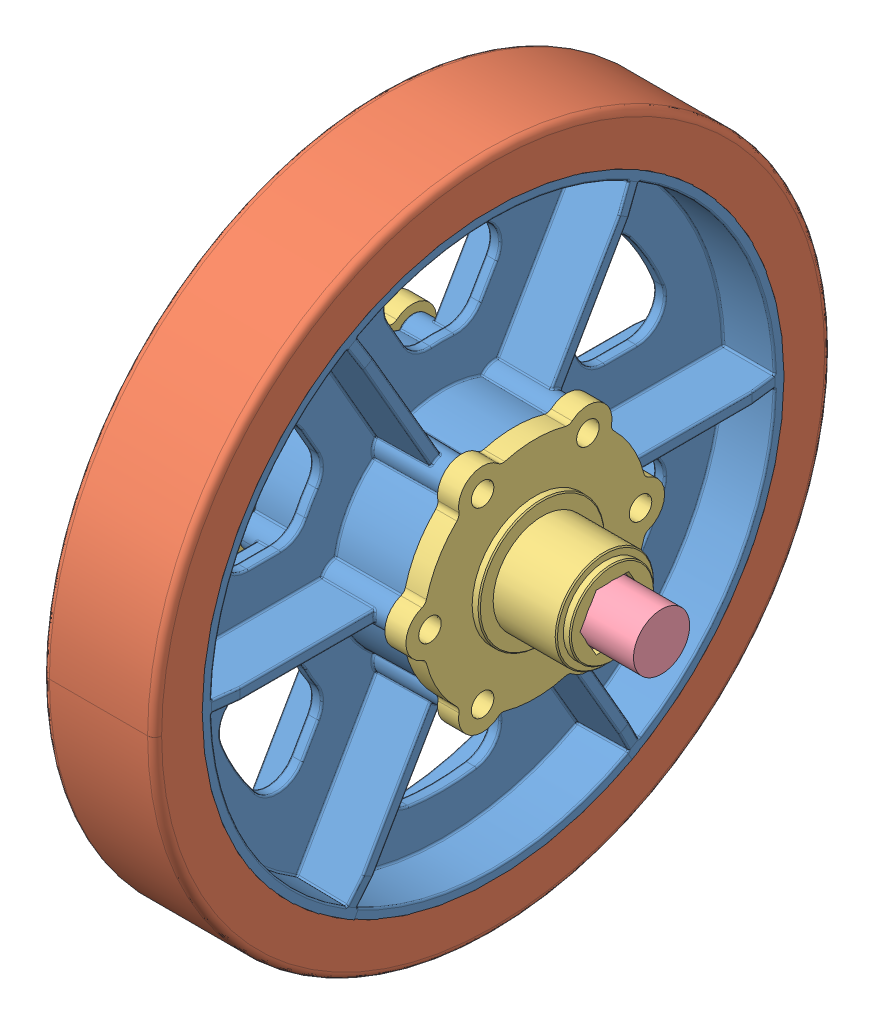
SolidWorks assembly 6in_wheel_assem, configuration Default. Lengths in mm.
Overall size (129.54 153.16 153.16).
6 component instances, 4 part files, 7 mates.
Components (placement in the parent):
- am-0144a SmoothGrip Wheel.STEP-1: am-0144a SmoothGrip Wheel.STEP [Default] at origin size (34.94 153.16 153.16)
  - 6 wheel Rev 4.STEP-1: 6 wheel Rev 4.STEP [Default] at origin
  - SmoothGrip Tread.STEP-1: SmoothGrip Tread.STEP [Default] x (0 0 1) z (-1 0 0)
- am-4124 500 Hex Hub-1: am-4124 500 Hex Hub [Default] at (-22.225 -26.0832 -29.2735) x (0 0 1) z (-1 0 0)
- 4416T651_Easy-to-Machine 1215 Carbon Steel-1: 4416T651_Easy-to-Machine 1215 Carbon Steel [4416T651] x (0 -0.5 -0.866025) z (1 0 0)
- am-4124 500 Hex Hub-2: am-4124 500 Hex Hub [Default] at (22.225 26.0832 -29.2735) x (0 0 1) z (1 0 0)
Mates (geometry in assembly coordinates):
- Concentric1: concentric aligned: cone of am-0144a SmoothGrip Wheel.STEP-1/6 wheel Rev 4.STEP-1 through (0 0 0) axis (1 0 0); cylinder of am-4124 500 Hex Hub-1 through (-38.1 0 0) axis (1 0 0) radius 11.1125
- Concentric2: concentric anti-aligned: cylinder of am-0144a SmoothGrip Wheel.STEP-1/6 wheel Rev 4.STEP-1 through (17.4625 20.6222 -11.9062) axis (-1 0 0) radius 1.9939; cylinder of am-4124 500 Hex Hub-1 through (-22.225 20.6222 -11.9062) axis (1 0 0) radius 2.5527
- Coincident1: coincident anti-aligned: plane of am-0144a SmoothGrip Wheel.STEP-1/6 wheel Rev 4.STEP-1 through (-17.4625 0 0) normal (-1 0 0); plane of am-4124 500 Hex Hub-1 through (-17.4625 10.3111 5.9531) normal (1 0 0)
- Coincident2: coordinate: point of am-0144a SmoothGrip Wheel.STEP-1
- Concentric3: concentric anti-aligned: cylinder of am-4124 500 Hex Hub-1 through (-38.1 0 0) axis (1 0 0) radius 11.1125; line of 4416T651_Easy-to-Machine 1215 Carbon Steel-1 through (167.64 0 0) axis (-1 0 0)
- Parallel1: parallel anti-aligned: plane of am-4124 500 Hex Hub-1 through (-39.6875 6.35 -3.6662) normal (0 -1 0); plane of 4416T651_Easy-to-Machine 1215 Carbon Steel-1 through (53.975 6.35 -3.6662) normal (0 1 0)
- Coincident4: coincident aligned: plane of 4416T651_Easy-to-Machine 1215 Carbon Steel-1 through (0 0 0) normal (1 0 0)
